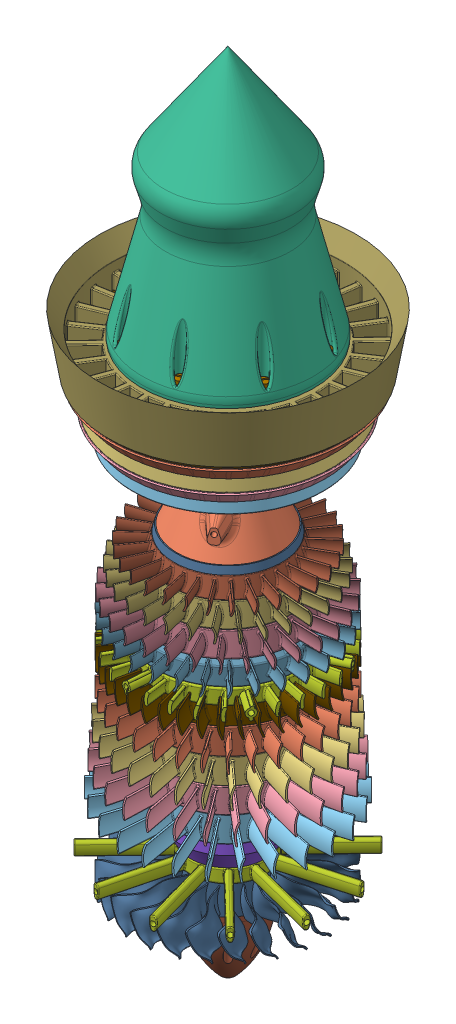
SolidWorks assembly Main Axis Assembly, configuration Default. Lengths in mm.
Overall size (446.53 812.06 446.53).
126 component instances, 45 part files, 38 mates.
Components (placement in the parent):
- Main Axis Shaft-1: Main Axis Shaft [Default] at (269.3467 22.5392 446.4756) size (36 615.58 36)
- Core-1: Core [Default] at (269.3467 438.4586 446.4756) x (0 -1 0) z (-0.809663 0 0.586895) size (71.31 135.2 135.2)
- Core Plate-1: Core Plate [Default] at (269.3467 392.7556 446.4756) x (0.950716 0 0.310062) z (-0.310062 0 0.950716) size (74 6.57 74)
- Turbine shaft-1: Turbine shaft [Default] at (269.3467 445.0933 446.4756) x (0.233986 0 0.97224) z (-0.97224 0 0.233986) size (66 109.5 66)
- hex nut structural gradeb 10_iso-1: hex nut structural gradeb 10_iso [Hexagon Nut ISO - 7414 - M22 - W - N] at (269.3467 335.4802 446.4756) x (1 0 0) z (0 1 0) size (36 41.57 19.4)
- socket countersunk head screw_iso-1: socket countersunk head screw_iso [ISO 10642 - M6 x 25 - 25N] at (275.1964 351.5633 470.7816) x (0 -1 0) z (-0.546944 0 0.837169) size (25 11.34 11.34)
- socket countersunk head screw_iso-2: socket countersunk head screw_iso [ISO 10642 - M6 x 25 - 25N] at (248.038 351.5633 459.5499) x (0 -1 0) z (-0.96521 0 -0.261475) size (25 11.34 11.34)
- socket countersunk head screw_iso-3: socket countersunk head screw_iso [ISO 10642 - M6 x 25 - 25N] at (250.3276 351.5633 430.2499) x (0 -1 0) z (-0.049589 0 -0.99877) size (25 11.34 11.34)
- socket countersunk head screw_iso-4: socket countersunk head screw_iso [ISO 10642 - M6 x 25 - 25N] at (278.901 351.5633 423.3733) x (0 -1 0) z (0.934563 0 -0.355798) size (25 11.34 11.34)
- socket countersunk head screw_iso-5: socket countersunk head screw_iso [ISO 10642 - M6 x 25 - 25N] at (294.2708 351.5633 448.4232) x (0 -1 0) z (0.62718 0 0.778874) size (25 11.34 11.34)
- socket countersunk head screw_iso-7: socket countersunk head screw_iso [ISO 10642 - M4 x 16 - 16N] at (259.4247 389.9526 476.8985) x (0 1 0) z (-0.777692 0 -0.628645) size (16 7.53 7.53)
- socket countersunk head screw_iso-8: socket countersunk head screw_iso [ISO 10642 - M4 x 16 - 16N] at (295.2146 389.9526 465.3131) x (0 1 0) z (-0.838197 0 0.545367) size (16 7.53 7.53)
- socket countersunk head screw_iso-9: socket countersunk head screw_iso [ISO 10642 - M4 x 16 - 16N] at (295.2559 389.9526 427.6949) x (0 1 0) z (0.259658 0 0.965701) size (16 7.53 7.53)
- socket countersunk head screw_iso-10: socket countersunk head screw_iso [ISO 10642 - M4 x 16 - 16N] at (259.4917 389.9526 416.0309) x (0 1 0) z (0.998675 0 0.051469) size (16 7.53 7.53)
- socket countersunk head screw_iso-11: socket countersunk head screw_iso [ISO 10642 - M4 x 16 - 16N] at (237.3468 389.9526 446.4404) x (0 1 0) z (0.357557 0 -0.933891) size (16 7.53 7.53)
- Rear Compression Structure-2: Rear Compression Structure [Default] at (269.3467 262.8802 446.4756) x (0 1 0) z (-0.085691 0 0.996322) size (27 190 190)
- Mid Compression Cap-1: Mid Compression Cap [Default] at (269.3467 269.8802 446.4756) x (0.996322 0 0.085691) z (0.085691 0 -0.996322) size (91 11 91)
- socket head cap screw_iso-1: socket head cap screw_iso [ISO 4762 M5 x 8 - 8N] at (266.3475 258.8802 481.3468) x (0 1 0) z (-0.509631 0 -0.860393) size (13 8.5 8.5)
- socket head cap screw_iso-2: socket head cap screw_iso [ISO 4762 M5 x 8 - 8N] at (291.8837 258.8802 473.254) x (0 1 0) z (-0.968753 0 -0.248027) size (13 8.5 8.5)
- socket head cap screw_iso-3: socket head cap screw_iso [ISO 4762 M5 x 8 - 8N] at (304.218 258.8802 449.4748) x (0 1 0) z (-0.860393 0 0.509631) size (13 8.5 8.5)
- socket head cap screw_iso-4: socket head cap screw_iso [ISO 4762 M5 x 8 - 8N] at (296.1252 258.8802 423.9386) x (0 1 0) z (-0.248027 0 0.968753) size (13 8.5 8.5)
- socket head cap screw_iso-5: socket head cap screw_iso [ISO 4762 M5 x 8 - 8N] at (272.3459 258.8802 411.6043) x (0 1 0) z (0.509631 0 0.860393) size (13 8.5 8.5)
- socket head cap screw_iso-6: socket head cap screw_iso [ISO 4762 M5 x 8 - 8N] at (246.8098 258.8802 419.6971) x (0 1 0) z (0.968753 0 0.248027) size (13 8.5 8.5)
- socket head cap screw_iso-7: socket head cap screw_iso [ISO 4762 M5 x 8 - 8N] at (234.4755 258.8802 443.4764) x (0 1 0) z (0.860393 0 -0.509631) size (13 8.5 8.5)
- socket head cap screw_iso-8: socket head cap screw_iso [ISO 4762 M5 x 8 - 8N] at (242.5683 258.8802 469.0125) x (0 1 0) z (0.248027 0 -0.968753) size (13 8.5 8.5)
- Rear Compression Assembly-1: Rear Compression Assembly [Default] at (266.4206 428.995 546.894) x (0.997836 0 0.065753) z (0.065753 0 -0.997836) size (266.35 92.17 266.35)
  - Mid Axis Cover-1: Mid Axis Cover [Default] at (-3.683 58.4458 100.3935) size (108.6 15 108.6)
  - Rear Compression Fan 1-1: Rear Compression Fan 1 [Default] at (-3.683 84.4458 100.3935) x (0.939693 0 -0.34202) z (-0.34202 0 -0.939693) size (165 19 165)
  - Rear Compression Fan 2-1: Rear Compression Fan 2 [Default] at (-3.683 105.9458 100.3935) x (0.19125 0 -0.981541) z (-0.981541 0 -0.19125) size (177.5 21.5 177.5)
  - Rear Compression Fan 3-1: Rear Compression Fan 3 [Default] at (-3.683 131.3458 100.3935) x (-0.763784 0 0.645472) z (0.645472 0 0.763784) size (189 22.06 189)
  - Mid Compression Fan-1: Mid Compression Fan [Default] at (-3.683 150.6148 100.3935) x (0.373154 0 0.927769) z (0.927769 0 -0.373154) size (190 26 190)
  - Rear Compression Hub-1: Rear Compression Hub [Default] at (-3.683 140.1148 100.3935) x (0.968402 0 0.249393) z (0.249393 0 -0.968402) size (108 26 108)
  - Rear Compression Link-1: Rear Compression Link [Default] at (7.7207 63.1148 57.8344) x (0.985834 0 -0.167725) z (0.167725 0 0.985834) size (12 68 12)
  - Rear Compression Link-2: Rear Compression Link [Default] at (40.317 63.1148 98.0876) x (0.464155 0 0.885754) z (-0.885754 0 0.464155) size (12 68 12)
  - Rear Compression Link-3: Rear Compression Link [Default] at (12.1068 63.1148 141.5274) x (-0.69897 0 0.715151) z (-0.715151 0 -0.69897) size (12 68 12)
  - Rear Compression Link-4: Rear Compression Link [Default] at (-37.9244 63.1148 128.1216) x (-0.896142 0 -0.443767) z (0.443767 0 -0.896142) size (12 68 12)
  - Rear Compression Link-5: Rear Compression Link [Default] at (-40.6352 63.1148 76.3965) x (0.145124 0 -0.989414) z (0.989414 0 0.145124) size (12 68 12)
  - socket countersunk head screw_iso-1: socket countersunk head screw_iso [ISO 10642 - M6 x 25 - 25N] at (-40.6352 58.4458 76.3965) x (0 1 0) z (-0.035554 0 0.999368) size (25 11.34 11.34)
  - socket countersunk head screw_iso-2: socket countersunk head screw_iso [ISO 10642 - M6 x 25 - 25N] at (7.7207 58.4458 57.8344) x (0 1 0) z (-0.961442 0 0.275008) size (25 11.34 11.34)
  - socket countersunk head screw_iso-3: socket countersunk head screw_iso [ISO 10642 - M6 x 25 - 25N] at (40.317 58.4458 98.0876) x (0 1 0) z (-0.55865 0 -0.829404) size (25 11.34 11.34)
  - socket countersunk head screw_iso-4: socket countersunk head screw_iso [ISO 10642 - M6 x 25 - 25N] at (12.1068 58.4458 141.5274) x (0 1 0) z (0.616177 0 -0.787607) size (25 11.34 11.34)
  - socket countersunk head screw_iso-5: socket countersunk head screw_iso [ISO 10642 - M6 x 25 - 25N] at (-37.9244 58.4458 128.1216) x (0 1 0) z (0.939468 0 0.342635) size (25 11.34 11.34)
  - socket countersunk head screw_iso-6: socket countersunk head screw_iso [ISO 10642 - M6 x 25 - 25N] at (-40.8163 141.8348 76.7902) x (0 -1 0) z (0.690355 0 -0.723471) size (25 11.34 11.34)
  - socket countersunk head screw_iso-7: socket countersunk head screw_iso [ISO 10642 - M6 x 25 - 25N] at (-37.6059 141.8348 128.4155) x (0 -1 0) z (-0.47473 0 -0.880131) size (25 11.34 11.34)
  - socket countersunk head screw_iso-8: socket countersunk head screw_iso [ISO 10642 - M6 x 25 - 25N] at (12.4848 141.8348 141.3154) x (0 -1 0) z (-0.983754 0 0.17952) size (25 11.34 11.34)
  - socket countersunk head screw_iso-9: socket countersunk head screw_iso [ISO 10642 - M6 x 25 - 25N] at (40.2322 141.8348 97.6626) x (0 -1 0) z (-0.133264 0 0.991081) size (25 11.34 11.34)
  - socket countersunk head screw_iso-10: socket countersunk head screw_iso [ISO 10642 - M6 x 25 - 25N] at (7.2903 141.8348 57.7838) x (0 -1 0) z (0.901393 0 0.433002) size (25 11.34 11.34)
- Mid Compression Assembly-1: Mid Compression Assembly [Default] at (276.2527 278.8402 580.349) x (0.994711 0 -0.102714) z (-0.102714 0 -0.994711) size (258.32 160 258.32)
  - Rear Compression shaft-1: Rear Compression shaft [Default] at (6.8812 10.96 133.8747) size (100 148 100)
  - Compression Fan 1-1: Compression Fan 1 [Default] at (6.8812 4.96 133.8747) x (0.309017 0 -0.951057) z (0.951057 0 0.309017) size (190 30 190)
  - Mid Compression Link-1: Mid Compression Link [Default] at (17.6968 20.96 100.5877) x (0.336833 0 -0.941565) z (0.941565 0 0.336833) size (12 136 12)
  - Mid Compression Link-2: Mid Compression Link [Default] at (41.8812 20.96 133.8747) x (0.999568 0 0.029388) z (-0.029388 0 0.999568) size (12 136 12)
  - Mid Compression Link-3: Mid Compression Link [Default] at (17.6968 20.96 167.1617) x (0.280934 0 0.959727) z (-0.959727 0 0.280934) size (12 136 12)
  - Mid Compression Link-4: Mid Compression Link [Default] at (-21.4344 20.96 154.4472) x (-0.825941 0 0.563756) z (-0.563756 0 -0.825941) size (12 136 12)
  - Mid Compression Link-5: Mid Compression Link [Default] at (-21.4344 20.96 113.3022) x (-0.791394 0 -0.611306) z (0.611306 0 -0.791394) size (12 136 12)
  - Front Compression Fan 1-1: Front Compression Fan 1 [Default] at (6.8812 34.96 133.8747) x (0.951057 0 0.309017) z (-0.309017 0 0.951057) size (190 30 190)
  - Front Compression Fan 2-1: Front Compression Fan 2 [Default] at (6.8812 64.96 133.8747) x (0.951057 0 0.309017) z (-0.309017 0 0.951057) size (195 30 195)
  - Front Compression Fan 3-1: Front Compression Fan 3 [Default] at (6.8812 94.96 133.8747) x (0.951057 0 0.309017) z (-0.309017 0 0.951057) size (200 30 200)
  - Front Compression Fan 4-1: Front Compression Fan 4 [Default] at (6.8812 124.96 133.8747) x (0.951057 0 0.309017) z (-0.309017 0 0.951057) size (205 30 205)
  - Front Compression Hub-1: Front Compression Hub [Default] at (6.8812 164.96 133.8747) x (-0.309017 0 -0.951057) z (-0.951057 0 0.309017) size (90 10 90)
  - socket countersunk head screw_iso-1: socket countersunk head screw_iso [ISO 10642 - M6 x 25 - 25N] at (17.6968 10.96 100.5877) x (0 1 0) z (-0.308709 0 0.951157) size (25 11.34 11.34)
  - socket countersunk head screw_iso-2: socket countersunk head screw_iso [ISO 10642 - M6 x 25 - 25N] at (41.8812 10.96 133.8747) x (0 1 0) z (-1 0 0.000324) size (25 11.34 11.34)
  - socket countersunk head screw_iso-3: socket countersunk head screw_iso [ISO 10642 - M6 x 25 - 25N] at (17.6968 10.96 167.1617) x (0 1 0) z (-0.309325 0 -0.950956) size (25 11.34 11.34)
  - socket countersunk head screw_iso-4: socket countersunk head screw_iso [ISO 10642 - M6 x 25 - 25N] at (-21.4344 10.96 154.4472) x (0 1 0) z (0.808826 0 -0.588048) size (25 11.34 11.34)
  - socket countersunk head screw_iso-5: socket countersunk head screw_iso [ISO 10642 - M6 x 25 - 25N] at (-21.4344 10.96 113.3022) x (0 1 0) z (0.809208 0 0.587523) size (25 11.34 11.34)
  - socket countersunk head screw_iso-6: socket countersunk head screw_iso [ISO 10642 - M6 x 25 - 25N] at (17.6968 164.68 100.5877) x (0 -1 0) z (0.984101 0 0.17761) size (25 11.34 11.34)
  - socket countersunk head screw_iso-7: socket countersunk head screw_iso [ISO 10642 - M6 x 25 - 25N] at (-21.4344 164.68 113.3022) x (0 -1 0) z (0.473021 0 -0.881051) size (25 11.34 11.34)
  - socket countersunk head screw_iso-8: socket countersunk head screw_iso [ISO 10642 - M6 x 25 - 25N] at (-21.4344 164.68 154.4472) x (0 -1 0) z (-0.691758 0 -0.72213) size (25 11.34 11.34)
  - socket countersunk head screw_iso-9: socket countersunk head screw_iso [ISO 10642 - M6 x 25 - 25N] at (17.6968 164.68 167.1617) x (0 -1 0) z (-0.900551 0 0.434751) size (25 11.34 11.34)
  - socket countersunk head screw_iso-10: socket countersunk head screw_iso [ISO 10642 - M6 x 25 - 25N] at (41.8812 164.68 133.8747) x (0 -1 0) z (0.135187 0 0.99082) size (25 11.34 11.34)
- Intake Structure-1: Intake Structure [Default] at (269.3467 80.8802 446.4756) x (0.962139 0 -0.27256) z (0.27256 0 0.962139) size (220.24 15.04 220.24)
- Front Compression Cap-1: Front Compression Cap [Default] at (269.3467 95.8802 446.4756) x (-0.27256 0 -0.962139) z (-0.962139 0 0.27256) size (96 31 96)
- torque nut 03_iso-1: torque nut 03_iso [ISO 7042-M14-N] at (269.3467 36.7802 446.4756) x (0.290623 0 -0.956838) z (0 -1 0) size (22.61 25.86 14.1)
- Intake Fan-1: Intake Fan [Default] at (269.3467 50.8802 446.4756) x (0 0 1) z (-1 0 0) size (193.05 30.9 192.93)
- Nose Cone-1: Nose Cone [Default] at (269.3467 50.8802 446.4756) x (-0.707107 0 -0.707107) z (-0.707107 0 0.707107) size (70 75 70)
- Turbine Assembly-1: Turbine Assembly [Default] at (389.6401 680.7757 251.0115) x (-0.899408 0 -0.43711) z (-0.43711 0 0.899408) size (334.1 349.82 334.1)
  - Turbine Fan 1-1: Turbine Fan 1 [Default] at (22.7534 150.4171 228.3834) size (259 53.75 259)
  - needle roller bearing_nrba_iso-2: needle roller bearing_nrba_iso [ISO 1206-A - 493555 - 26,SI,NC,26] at (22.7534 136.5971 228.3834) x (0 -1 0) z (-0.182779 0 0.983154) size (20 55 55)
  - Rear Turbine Hub-2: Rear Turbine Hub [Default] at (22.7534 170.4171 228.3834) x (-0.970998 0 0.239087) z (0 1 0) size (101.62 104.75 40.92)
  - Turbine Link Assembly-1: Turbine Link Assembly [Default] at (-63.4742 236.9911 264.9834) x (0.691338 0 0.722532) z (0.722532 0 -0.691338) size (16 64.44 16)
    - Turbine Link-1: Turbine Link [Default] at (-7.9109 -2.865 69.2328) size (12 64.44 12)
    - Turbine Spacer 2-1: Turbine Spacer 2 [Default] at (-7.9109 3.135 69.2328) size (16 21.23 16)
    - Turbine Spacer-1: Turbine Spacer [Default] at (-7.9109 30.963 69.2328) size (16 23.35 16)
  - Turbine Link Assembly-2: Turbine Link Assembly [Default] at (-38.7011 236.9911 157.6861) x (-0.473533 0 0.880776) z (0.880776 0 0.473533) size (16 64.44 16)
    - Turbine Link-1: Turbine Link [Default] at (-7.9109 -2.865 69.2328) size (12 64.44 12)
    - Turbine Spacer 2-1: Turbine Spacer 2 [Default] at (-7.9109 3.135 69.2328) size (16 21.23 16)
    - Turbine Spacer-1: Turbine Spacer [Default] at (-7.9109 30.963 69.2328) size (16 23.35 16)
  - Turbine Link Assembly-3: Turbine Link Assembly [Default] at (71 236.9911 148.09) x (-0.983998 0 -0.178182) z (-0.178182 0 0.983998) size (16 64.44 16)
    - Turbine Link-1: Turbine Link [Default] at (-7.9109 -2.865 69.2328) size (12 64.44 12)
    - Turbine Spacer 2-1: Turbine Spacer 2 [Default] at (-7.9109 3.135 69.2328) size (16 21.23 16)
    - Turbine Spacer-1: Turbine Spacer [Default] at (-7.9109 30.963 69.2328) size (16 23.35 16)
  - Turbine Link Assembly-4: Turbine Link Assembly [Default] at (114.026 236.9911 249.4566) x (-0.134611 0 -0.990899) z (-0.990899 0 0.134611) size (16 64.44 16)
    - Turbine Link-1: Turbine Link [Default] at (-7.9109 -2.865 69.2328) size (12 64.44 12)
    - Turbine Spacer 2-1: Turbine Spacer 2 [Default] at (-7.9109 3.135 69.2328) size (16 21.23 16)
    - Turbine Spacer-1: Turbine Spacer [Default] at (-7.9109 30.963 69.2328) size (16 23.35 16)
  - Turbine Link Assembly-5: Turbine Link Assembly [Default] at (30.9163 236.9911 321.7007) x (0.900804 0 -0.434227) z (-0.434227 0 -0.900804) size (16 64.44 16)
    - Turbine Link-1: Turbine Link [Default] at (-7.9109 -2.865 69.2328) size (12 64.44 12)
    - Turbine Spacer 2-1: Turbine Spacer 2 [Default] at (-7.9109 3.135 69.2328) size (16 21.23 16)
    - Turbine Spacer-1: Turbine Spacer [Default] at (-7.9109 30.963 69.2328) size (16 23.35 16)
  - Turbine Fan 2-1: Turbine Fan 2 [Default] at (22.7534 165.4171 228.3834) x (-0.07267 0 0.997356) z (-0.997356 0 -0.07267) size (234 15.68 234)
  - Turbine Axis Spacer-1: Turbine Axis Spacer [Default] at (22.7534 234.8561 228.3834) x (0.984962 0 0.172768) z (0 -1 0) size (34 34 3)
  - Turbine Fan 5.-1: Turbine Fan 5. [Default] at (22.7534 200.4171 228.3834) x (0 1 0) z (0.739195 0 -0.673491) size (15.2 236.5 236.5)
  - Turbine Fan 3-2: Turbine Fan 3 [Default] at (22.7534 195.4171 228.3834) x (0.926086 0 0.377313) z (-0.377313 0 0.926086) size (212.5 14.22 212.5)
  - Turbine Fan 6-1: Turbine Fan 6 [Default] at (22.7534 226.9171 228.3834) x (0 1 0) z (0.881108 0 0.472915) size (13.18 215 215)
  - Turbine Fan 4-1: Turbine Fan 4 [Default] at (22.7534 233.9171 228.3834) x (0.926086 0 0.377313) z (0.377313 0 -0.926086) size (193 12.68 193)
  - Turbine Housing-1: Turbine Housing [Default] at (22.7534 -107.1644 228.3834) x (0 1 0) z (0 0 -1) size (257.58 181.79 181.21)
  - Front Turbine Hub-2: Front Turbine Hub [Default] at (22.7534 160.4171 228.3834) x (-0.07267 0 0.997356) z (0 1 0) size (101.62 104.75 10)
  - hex screw gradeab_iso-2: hex screw gradeab_iso [ISO 4017 - M4 x 8-N] at (66.4483 157.6171 217.6245) x (0 1 0) z (-0.789962 0 -0.613155) size (10.8 8.08 7)
  - hex screw gradeab_iso-3: hex screw gradeab_iso [ISO 4017 - M4 x 8-N] at (46.4882 157.6171 266.615) x (0 1 0) z (0.339034 0 -0.940774) size (10.8 8.08 7)
  - hex screw gradeab_iso-4: hex screw gradeab_iso [ISO 4017 - M4 x 8-N] at (-6.2726 157.6171 262.7707) x (0 1 0) z (0.999497 0 0.031725) size (10.8 8.08 7)
  - hex screw gradeab_iso-5: hex screw gradeab_iso [ISO 4017 - M4 x 8-N] at (-18.9204 157.6171 211.4043) x (0 1 0) z (0.278689 0 0.960381) size (10.8 8.08 7)
  - hex screw gradeab_iso-6: hex screw gradeab_iso [ISO 4017 - M4 x 8-N] at (26.0236 157.6171 183.5023) x (0 1 0) z (-0.827257 0 0.561823) size (10.8 8.08 7)
  - Front Turbine Hub-3: Front Turbine Hub [Default] at (22.7534 238.9171 228.3834) x (-0.970998 0 0.239087) z (0 -1 0) size (101.62 104.75 10)
  - slotted capstan screw_din-2: slotted capstan screw_din [DIN 404 M6 x 8 --- 8N] at (-55.2466 131.9671 228.3834) x (0 1 0) z (0 0 -1) size (16.43 10 10)
  - slotted capstan screw_din-4: slotted capstan screw_din [DIN 404 M6 x 8 --- 8N] at (-32.4009 131.9671 283.5377) x (0 1 0) z (-0.707107 0 -0.707107) size (16.43 10 10)
  - slotted capstan screw_din-5: slotted capstan screw_din [DIN 404 M6 x 8 --- 8N] at (22.7534 131.9671 306.3834) x (0 1 0) z (-1 0 0) size (16.43 10 10)
  - slotted capstan screw_din-6: slotted capstan screw_din [DIN 404 M6 x 8 --- 8N] at (77.9078 131.9671 283.5377) x (0 1 0) z (-0.707107 0 0.707107) size (16.43 10 10)
  - slotted capstan screw_din-7: slotted capstan screw_din [DIN 404 M6 x 8 --- 8N] at (100.7534 131.9671 228.3834) x (0 1 0) z (0 0 1) size (16.43 10 10)
  - slotted capstan screw_din-8: slotted capstan screw_din [DIN 404 M6 x 8 --- 8N] at (77.9078 131.9671 173.229) x (0 1 0) z (0.707107 0 0.707107) size (16.43 10 10)
  - slotted capstan screw_din-9: slotted capstan screw_din [DIN 404 M6 x 8 --- 8N] at (22.7534 131.9671 150.3834) x (0 1 0) z (1 0 0) size (16.43 10 10)
  - slotted capstan screw_din-10: slotted capstan screw_din [DIN 404 M6 x 8 --- 8N] at (-32.4009 131.9671 173.229) x (0 1 0) z (0.707107 0 -0.707107) size (16.43 10 10)
  - hex screw gradeab_iso-7: hex screw gradeab_iso [ISO 4017 - M4 x 8-N] at (26.0236 242.6561 183.5023) x (0 -1 0) z (0.122239 0 0.992501) size (10.8 8.08 7)
  - hex screw gradeab_iso-8: hex screw gradeab_iso [ISO 4017 - M4 x 8-N] at (-18.9204 242.6561 211.4043) x (0 -1 0) z (0.981698 0 0.190443) size (10.8 8.08 7)
  - hex screw gradeab_iso-9: hex screw gradeab_iso [ISO 4017 - M4 x 8-N] at (-6.2726 242.6561 262.7707) x (0 -1 0) z (0.484484 0 -0.8748) size (10.8 8.08 7)
  - hex screw gradeab_iso-10: hex screw gradeab_iso [ISO 4017 - M4 x 8-N] at (46.4882 242.6561 266.615) x (0 -1 0) z (-0.682271 0 -0.731099) size (10.8 8.08 7)
  - hex screw gradeab_iso-11: hex screw gradeab_iso [ISO 4017 - M4 x 8-N] at (66.4483 242.6561 217.6245) x (0 -1 0) z (-0.90615 0 0.422956) size (10.8 8.08 7)
Mates (geometry in assembly coordinates):
- Concentric1: concentric anti-aligned: cylinder of Main Axis Shaft-1 through (269.3467 469.3802 446.4756) axis (0 -1 0) radius 11; cylinder of Core-1 through (269.3467 438.4586 446.4756) axis (0 1 0) radius 15.5
- Concentric3: concentric aligned: cylinder of Main Axis Shaft-1 through (269.3467 469.3802 446.4756) axis (0 -1 0) radius 11; cylinder of Core Plate-1 through (269.3467 395.5586 446.4756) axis (0 -1 0) radius 15.5
- Coincident2: coincident anti-aligned: plane of Core-1 through (299.3043 395.5586 424.7604) normal (0 -1 0); plane of Core Plate-1 through (269.3467 395.5586 446.4756) normal (0 1 0)
- Concentric4: concentric aligned: cylinder of Core-1 through (259.4917 395.5586 416.0309) axis (0 -1 0) radius 1.61; cylinder of Core Plate-1 through (259.4917 390.6676 416.0309) axis (0 -1 0) radius 2.0585
- Concentric5: concentric anti-aligned: cylinder of Main Axis Shaft-1 through (269.3467 469.3802 446.4756) axis (0 -1 0) radius 11; cylinder of Turbine shaft-1 through (269.3467 445.0933 446.4756) axis (0 1 0) radius 13.566
- Concentric8: concentric anti-aligned: cylinder of Main Axis Shaft-1 through (269.3467 469.3802 446.4756) axis (0 -1 0) radius 11; cylinder of hex nut structural gradeb 10_iso-1 through (269.3467 316.0802 446.4756) axis (0 1 0) radius 9.75
- Coincident4: coincident anti-aligned: plane of Main Axis Shaft-1 through (269.3467 316.0802 446.4756) normal (0 1 0); plane of hex nut structural gradeb 10_iso-1 through (233.3467 316.0802 446.4756) normal (0 -1 0)
- Concentric9: concentric aligned: cylinder of Turbine shaft-1 through (275.1964 350.5433 470.7816) axis (0 1 0) radius 3; cylinder of socket countersunk head screw_iso-1 through (275.1964 351.5633 470.7816) axis (0 1 0) radius 3
- Coincident5: coincident aligned: cone of Turbine shaft-1 through (275.1964 350.5433 470.7816) axis (0 -1 0); cone of socket countersunk head screw_iso-1 through (275.1964 350.5133 470.7816) axis (0 -1 0)
- Concentric10: concentric aligned: cylinder of Core Plate-1 through (259.4247 390.6676 476.8985) axis (0 -1 0) radius 2.0585; cylinder of socket countersunk head screw_iso-7 through (259.4247 389.9526 476.8985) axis (0 -1 0) radius 2
- Concentric12: concentric aligned: cylinder of Main Axis Shaft-1 through (269.3467 282.3802 446.4756) axis (0 -1 0) radius 15; cylinder of Rear Compression Structure-2 through (269.3467 287.8802 446.4756) axis (0 -1 0) radius 27.5
- Coincident7: coincident aligned: plane of Main Axis Shaft-1 through (269.3467 288.3802 446.4756) normal (0 1 0); plane of Rear Compression Structure-2 through (246.8098 288.3802 419.6971) normal (0 1 0)
- Concentric13: concentric aligned: cylinder of Main Axis Shaft-1 through (269.3467 256.5392 446.4756) axis (0 -1 0) radius 10; cylinder of Mid Compression Cap-1 through (269.3467 258.8802 446.4756) axis (0 -1 0) radius 23
- Coincident8: coincident anti-aligned: plane of Rear Compression Structure-2 through (269.3467 267.8802 446.4756) normal (0 -1 0); plane of Mid Compression Cap-1 through (269.3467 267.8802 446.4756) normal (0 1 0)
- Concentric14: concentric aligned: cylinder of Rear Compression Structure-2 through (266.3475 288.3802 481.3468) axis (0 -1 0) radius 2.1; cylinder of Mid Compression Cap-1 through (266.3475 258.8802 481.3468) axis (0 -1 0) radius 2.75
- Concentric15: concentric aligned: cylinder of Mid Compression Cap-1 through (266.3475 258.8802 481.3468) axis (0 -1 0) radius 2.75; cylinder of socket head cap screw_iso-1 through (266.3475 227.1302 481.3468) axis (0 -1 0) radius 2.5
- Coincident9: coincident anti-aligned: plane of Mid Compression Cap-1 through (244.6723 263.8802 467.2417) normal (0 -1 0); plane of socket head cap screw_iso-1 through (270.0042 263.8802 479.1809) normal (0 1 0)
- Concentric16: concentric aligned: cylinder of Main Axis Shaft-1 through (269.3467 256.5392 446.4756) axis (0 -1 0) radius 10; cylinder of Rear Compression Assembly-1/Rear Compression Hub-1 through (269.3467 297.8802 446.4756) axis (0 -1 0) radius 54
- Coincident10: coincident anti-aligned: plane of Rear Compression Structure-2 through (269.3467 278.3802 446.4756) normal (0 1 0); plane of Rear Compression Assembly-1/Mid Compression Fan-1 through (269.3467 278.3802 446.4756) normal (0 -1 0)
- Coincident11: coincident aligned: cone of Core Plate-1 through (237.3468 390.6676 446.4404) axis (0 1 0); cone of socket countersunk head screw_iso-11 through (237.3468 390.6676 446.4404) axis (0 1 0)
- Coincident12: coincident anti-aligned: plane of Core-1 through (311.005 370.5492 416.279) normal (0 -1 0); plane of Rear Compression Assembly-1/Mid Axis Cover-1 through (269.3467 370.5492 446.4756) normal (0 1 0)
- Concentric17: concentric aligned: cylinder of Main Axis Shaft-1 through (269.3467 256.5392 446.4756) axis (0 -1 0) radius 10; cylinder of Mid Compression Assembly-1/Front Compression Hub-1 through (269.3467 123.8802 446.4756) axis (0 -1 0) radius 10
- Coincident13: coincident anti-aligned: plane of Rear Compression Structure-2 through (269.3467 267.8802 446.4756) normal (0 -1 0); plane of Mid Compression Assembly-1/Compression Fan 1-1 through (269.3467 267.8802 446.4756) normal (0 1 0)
- Concentric18: concentric aligned: cylinder of Main Axis Shaft-1 through (269.3467 102.5392 446.4756) axis (0 -1 0) radius 8.5; cylinder of Intake Structure-1 through (269.3467 95.8802 446.4756) axis (0 -1 0) radius 20
- Concentric19: concentric aligned: cylinder of Main Axis Shaft-1 through (269.3467 102.5392 446.4756) axis (0 -1 0) radius 8.5; cylinder of Front Compression Cap-1 through (269.3467 123.8802 446.4756) axis (0 -1 0) radius 10
- Coincident16: coincident anti-aligned: plane of Mid Compression Assembly-1/Front Compression Hub-1 through (269.3467 113.8802 446.4756) normal (0 -1 0); plane of Front Compression Cap-1 through (259.1257 113.8802 410.3954) normal (0 1 0)
- Concentric20: concentric anti-aligned: cylinder of Intake Structure-1 through (261.9876 80.8802 420.4978) axis (0 -1 0) radius 2.75; cylinder of Front Compression Cap-1 through (261.9876 113.8802 420.4978) axis (0 1 0) radius 2.1
- Coincident17: coincident anti-aligned: plane of Intake Structure-1 through (269.3467 95.8802 446.4756) normal (0 1 0); plane of Front Compression Cap-1 through (269.3467 95.8802 446.4756) normal (0 -1 0)
- Concentric21: concentric aligned: cylinder of Main Axis Shaft-1 through (269.3467 102.5392 446.4756) axis (0 -1 0) radius 8.5; cylinder of torque nut 03_iso-1 through (269.3467 50.8802 446.4756) axis (0 -1 0) radius 6
- Concentric22: concentric aligned: cylinder of Main Axis Shaft-1 through (269.3467 102.5392 446.4756) axis (0 -1 0) radius 8.5; cylinder of Intake Fan-1 through (269.3467 80.8802 446.4756) axis (0 -1 0) radius 8.5
- Coincident19: coincident anti-aligned: plane of Main Axis Shaft-1 through (263.3467 114.7926 440.4548) normal (0 0 -1); plane of Intake Fan-1 through (275.3467 80.8802 440.4548) normal (0 0 1)
- Coincident20: coincident anti-aligned: plane of Intake Structure-1 through (269.3467 80.8802 446.4756) normal (0 -1 0); plane of Intake Fan-1 through (269.3467 80.8802 446.4756) normal (0 1 0)
- Coincident21: coincident anti-aligned: plane of torque nut 03_iso-1 through (280.9478 50.8802 449.9992) normal (0 1 0); plane of Intake Fan-1 through (269.3467 50.8802 446.4756) normal (0 -1 0)
- Concentric23: concentric anti-aligned: cylinder of Intake Fan-1 through (269.3467 80.8802 446.4756) axis (0 -1 0) radius 35; cylinder of Nose Cone-1 through (269.3467 50.8802 446.4756) axis (0 1 0) radius 20
- Coincident22: coincident anti-aligned: plane of Intake Fan-1 through (269.3467 50.8802 446.4756) normal (0 -1 0); plane of Nose Cone-1 through (255.2046 50.8802 432.3334) normal (0 1 0)
- Concentric24: concentric aligned: cylinder of Intake Fan-1 through (289.1457 80.8802 466.2745) axis (0 1 0) radius 1.65; cylinder of Nose Cone-1 through (289.1457 50.8802 466.2745) axis (0 1 0) radius 2
- Concentric25: concentric aligned: cylinder of Main Axis Shaft-1 through (269.3467 608.1172 446.4756) axis (0 -1 0) radius 9; cylinder of Turbine Assembly-1/Turbine Fan 3-2 through (269.3467 485.9586 446.4756) axis (0 -1 0) radius 106.25
- Coincident25: coincident anti-aligned: plane of Core-1 through (269.3467 441.8586 446.4756) normal (0 1 0); plane of Turbine Assembly-1/Front Turbine Hub-3 through (269.3467 441.8586 446.4756) normal (0 -1 0)
